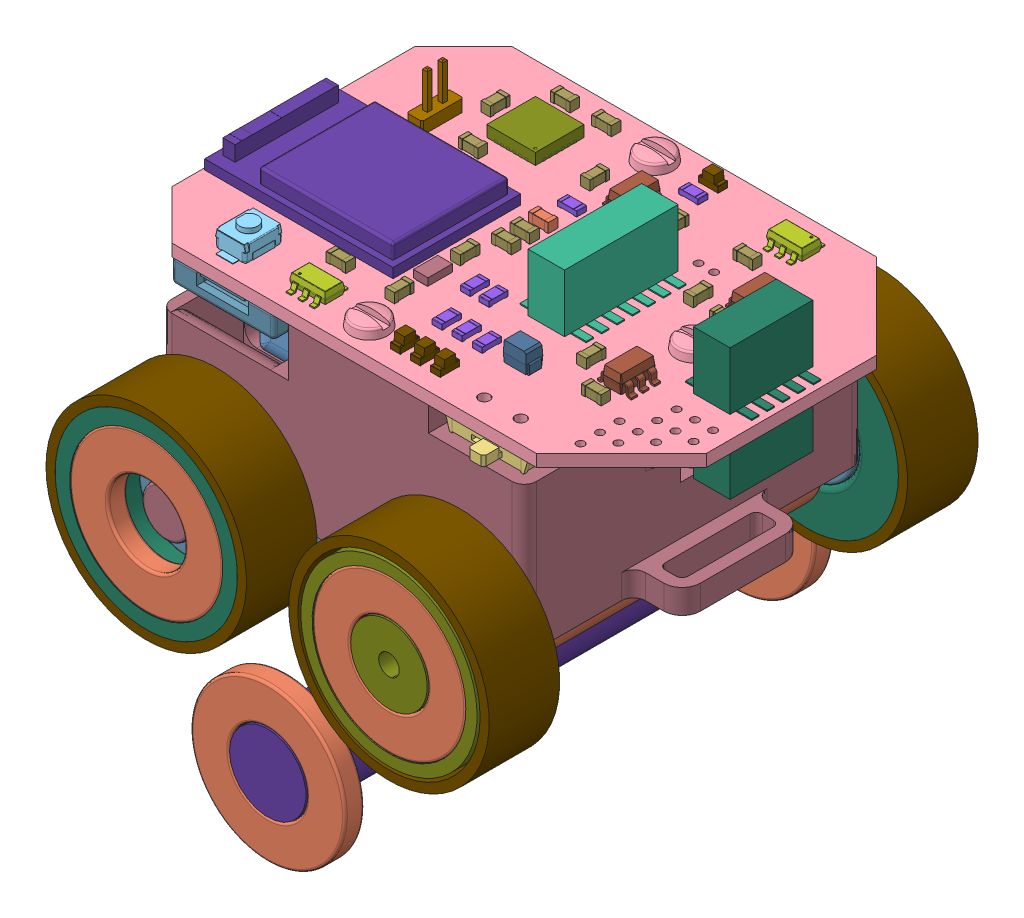
SolidWorks assembly AstroAnt_small_magnet, configuration Default. Lengths in mm.
Overall size (41.76 38.98 40.25).
158 component instances, 38 part files, 35 mates.
Components (placement in the parent):
- LiPo_360mAh-1: LiPo_360mAh [Default] at (6.8166 4.9998 44.2756) size (25 7 18)
- PA2-50-1: PA2-50 [Default] at (8.0673 -18.301 41.8029) x (0 0 1) z (0.952879 0.303349 0) size (29.1 8 8)
- PA2-50-2: PA2-50 [Default] at (-4.1563 19.5334 49.6029) x (0 0 -1) z (0.755989 -0.654584 0) size (29.1 8 8)
- 92120A150_Brass Heat-Set Inserts for Plastic-1: 92120A150_Brass Heat-Set Inserts for Plastic [92120A150] at (19.9543 12.4998 45.7029) size (2.56 3.33 2.56)
- 92120A150_Brass Heat-Set Inserts for Plastic-2: 92120A150_Brass Heat-Set Inserts for Plastic [92120A150] at (4.9543 12.4998 33.9529) size (2.56 3.33 2.56)
- 92120A150_Brass Heat-Set Inserts for Plastic-3: 92120A150_Brass Heat-Set Inserts for Plastic [92120A150] at (4.9543 12.4998 57.4529) size (2.56 3.33 2.56)
- 91460A005_METRIC CHEESE HEAD SLOTTED MACHINE SCREW-8: 91460A005_METRIC CHEESE HEAD SLOTTED MACHINE SCREW [91460A005] at (4.9543 14.9998 57.4529) x (1 0 0) z (0 1 0) size (3 3 7.1)
- 91460A005_METRIC CHEESE HEAD SLOTTED MACHINE SCREW-9: 91460A005_METRIC CHEESE HEAD SLOTTED MACHINE SCREW [91460A005] at (4.9543 14.9998 33.9529) x (1 0 0) z (0 1 0) size (3 3 7.1)
- 91460A005_METRIC CHEESE HEAD SLOTTED MACHINE SCREW-10: 91460A005_METRIC CHEESE HEAD SLOTTED MACHINE SCREW [91460A005] at (19.9543 14.9998 45.7029) x (1 0 0) z (0 1 0) size (3 3 7.1)
- 92120A150_Brass Heat-Set Inserts for Plastic-4: 92120A150_Brass Heat-Set Inserts for Plastic [92120A150] at (4.9543 1.4998 57.4529) x (-0.616962 0 -0.786993) z (0.786993 0 -0.616962) size (2.56 3.33 2.56)
- 92120A150_Brass Heat-Set Inserts for Plastic-5: 92120A150_Brass Heat-Set Inserts for Plastic [92120A150] at (4.9543 1.4998 33.9529) x (-0.616962 0 -0.786993) z (0.786993 0 -0.616962) size (2.56 3.33 2.56)
- 91460A005_METRIC CHEESE HEAD SLOTTED MACHINE SCREW-14: 91460A005_METRIC CHEESE HEAD SLOTTED MACHINE SCREW [91460A005] at (4.9543 -2.5002 57.4529) x (0.663599 0 0.748089) z (0 -1 0) size (3 3 7.1)
- 91460A005_METRIC CHEESE HEAD SLOTTED MACHINE SCREW-15: 91460A005_METRIC CHEESE HEAD SLOTTED MACHINE SCREW [91460A005] at (4.9543 -2.5002 33.9529) x (0.663599 0 0.748089) z (0 -1 0) size (3 3 7.1)
- mainboard_v1.step-1: mainboard_v1.step [Default] at (-103.0457 13.9998 235.7029) x (0 0 -1) z (0 1 0) size (29.41 41 10.8)
  - B3U-1000P.step-1: B3U-1000P.step [Default] at (178.95 -97.38 1.05) x (1 0 0) z (0 -1 0) size (4 1.75 2.5)
    - COMPOUND.step-1: COMPOUND.step [Default] at origin size (4 1.75 2.5)
  - 20021321-00014C1LF.step-1: 20021321-00014C1LF.step [Default] at (190 -115.5 1.05) size (9.35 5.45 4.85)
    - COMPOUND-0.step-1: COMPOUND-0.step [Default] at origin size (9.35 5.45 4.85)
  - MP6513GJ-Z.step-1: MP6513GJ-Z.step [Default] at (201.21 -120 1.05) x (-1 0 0) z (0 0 1) size (2.8 2.9 1)
    - COMPOUND-1.step-1: COMPOUND-1.step [Default] at origin size (2.8 2.9 1)
  - MP6513GJ-Z.step-2: MP6513GJ-Z.step [Default] at (178.51 -103.46 1.05) size (2.8 2.9 1)
    - COMPOUND-1.step-1: COMPOUND-1.step [Default] at origin size (2.8 2.9 1)
  - R_0603_1608Metric.step-1: R_0603_1608Metric.step [Default] at (195.55 -104.38 -0.05) x (1 0 0) z (0 0 -1) size (1.6 0.8 0.45)
    - SOLID.step-1: SOLID.step [Default] at origin size (1.6 0.8 0.45)
  - R_0603_1608Metric.step-2: R_0603_1608Metric.step [Default] at (192.6 -99.86 -0.05) x (0 1 0) z (0 0 -1) size (1.6 0.8 0.45)
    - SOLID.step-1: SOLID.step [Default] at origin size (1.6 0.8 0.45)
  - PinHeader_2x01_P1.27mm_Vertical.step-1: PinHeader_2x01_P1.27mm_Vertical.step [Default] at (194.96 -96.07 1.05) size (3.4 1.27 6.3)
    - SOLID-2.step-1: SOLID-2.step [Default] at origin size (3.4 1.27 6.3)
  - TAJP106K010RNJ.step-1: TAJP106K010RNJ.step [Default] at (196.22 -98.14 -0.05) x (-1 0 0) z (0 0 -1) size (2.05 1.4 1.7)
    - COMPOUND-3.step-1: COMPOUND-3.step [Default] at origin size (2.05 1.4 1.7)
  - TAJP106K010RNJ.step-2: TAJP106K010RNJ.step [Default] at (181.68 -117.23 1.05) x (0 1 0) z (0 0 1) size (2.05 1.4 1.7)
    - COMPOUND-3.step-1: COMPOUND-3.step [Default] at origin size (2.05 1.4 1.7)
  - SOT-23-5.step-1: SOT-23-5.step [Default] at (195.38 -122.78 1.05) x (0 1 0) z (0 0 1) size (2.8 2.9 1.55)
    - SOLID-4.step-1: SOLID-4.step [Default] at origin size (2.8 2.9 1.55)
  - C_0603_1608Metric.step-1: C_0603_1608Metric.step [Default] at (192.91 -122.55 1.05) x (0 -1 0) z (0 0 1) size (1.6 0.8 0.8)
    - SOLID-5.step-1: SOLID-5.step [Default] at origin size (1.6 0.8 0.8)
  - C_0603_1608Metric.step-2: C_0603_1608Metric.step [Default] at (193.57 -119.76 1.05) size (1.6 0.8 0.8)
    - SOLID-5.step-1: SOLID-5.step [Default] at origin size (1.6 0.8 0.8)
  - ECS-.327-12.5-12-TR.step-1: ECS-.327-12.5-12-TR.step [Default] at (184.31 -107.18 1.05) size (2 1.2 0.7)
    - COMPOUND-6.step-1: COMPOUND-6.step [Default] at origin size (2 1.2 0.7)
  - C_0603_1608Metric.step-3: C_0603_1608Metric.step [Default] at (197.67 -113.69 1.05) size (1.6 0.8 0.8)
    - SOLID-5.step-1: SOLID-5.step [Default] at origin size (1.6 0.8 0.8)
  - C_0603_1608Metric.step-4: C_0603_1608Metric.step [Default] at (197.64 -107.18 1.05) size (1.6 0.8 0.8)
    - SOLID-5.step-1: SOLID-5.step [Default] at origin size (1.6 0.8 0.8)
  - C_0603_1608Metric.step-5: C_0603_1608Metric.step [Default] at (190.96 -108.09 1.05) x (0 1 0) z (0 0 1) size (1.6 0.8 0.8)
    - SOLID-5.step-1: SOLID-5.step [Default] at origin size (1.6 0.8 0.8)
  - 1734592-6.step-1: 1734592-6.step [Default] at (203.79 -118 -1.05) x (0 -1 0) z (1 0 0) size (8.43 2.05 5.11)
    - SOLID-7.step-1: SOLID-7.step [Default] at origin size (8.43 2.05 5.11)
  - 1734592-6.step-2: 1734592-6.step [Default] at (176.19 -98 -1.05) x (0 1 0) z (-1 0 0) size (8.43 2.05 5.11)
    - SOLID-7.step-1: SOLID-7.step [Default] at origin size (8.43 2.05 5.11)
  - 20021321-00010C4LF.step-1: 20021321-00010C4LF.step [Default] at (190 -127.85 -0.05) x (1 0 0) z (0 0 -1) size (6.81 5.45 4.85)
    - COMPOUND-8.step-1: COMPOUND-8.step [Default] at origin size (6.81 5.45 4.85)
  - 20021321-00010C4LF.step-2: 20021321-00010C4LF.step [Default] at (190 -127.85 1.05) size (6.81 5.45 4.85)
    - COMPOUND-8.step-1: COMPOUND-8.step [Default] at origin size (6.81 5.45 4.85)
  - C_0603_1608Metric.step-6: C_0603_1608Metric.step [Default] at (181.31 -102.6 1.05) x (0 -1 0) z (0 0 1) size (1.6 0.8 0.8)
    - SOLID-5.step-1: SOLID-5.step [Default] at origin size (1.6 0.8 0.8)
  - C_0603_1608Metric.step-7: C_0603_1608Metric.step [Default] at (198.25 -119.14 1.05) x (0 -1 0) z (0 0 1) size (1.6 0.8 0.8)
    - SOLID-5.step-1: SOLID-5.step [Default] at origin size (1.6 0.8 0.8)
  - MPU6050.step-1: MPU6050.step [Default] at (198.43 -101.5 1.05) x (0 1 0) z (1 0 0) size (4 0.95 4)
    - COMPOUND-9.step-1: COMPOUND-9.step [Default] at origin size (4 0.95 4)
  - C_0603_1608Metric.step-8: C_0603_1608Metric.step [Default] at (194.9 -99.89 1.05) x (0 -1 0) z (0 0 1) size (1.6 0.8 0.8)
    - SOLID-5.step-1: SOLID-5.step [Default] at origin size (1.6 0.8 0.8)
  - C_0603_1608Metric.step-9: C_0603_1608Metric.step [Default] at (201.98 -100.38 1.05) x (0 -1 0) z (0 0 1) size (1.6 0.8 0.8)
    - SOLID-5.step-1: SOLID-5.step [Default] at origin size (1.6 0.8 0.8)
  - C_0603_1608Metric.step-10: C_0603_1608Metric.step [Default] at (201.98 -103.78 1.05) x (0 1 0) z (0 0 1) size (1.6 0.8 0.8)
    - SOLID-5.step-1: SOLID-5.step [Default] at origin size (1.6 0.8 0.8)
  - C_0603_1608Metric.step-11: C_0603_1608Metric.step [Default] at (198.81 -97.82 1.05) size (1.6 0.8 0.8)
    - SOLID-5.step-1: SOLID-5.step [Default] at origin size (1.6 0.8 0.8)
  - SOT-23-5.step-2: SOT-23-5.step [Default] at (184.86 -122.77 1.05) x (0 1 0) z (0 0 1) size (2.8 2.9 1.55)
    - SOLID-4.step-1: SOLID-4.step [Default] at origin size (2.8 2.9 1.55)
  - SOT-23-5.step-3: SOT-23-5.step [Default] at (197.58 -110.46 1.05) x (0 1 0) z (0 0 1) size (2.8 2.9 1.55)
    - SOLID-4.step-1: SOLID-4.step [Default] at origin size (2.8 2.9 1.55)
  - MDBT50Q-1MV2.step-1: MDBT50Q-1MV2.step [Default] at (187.3136 -98.605 1.0754) x (-1 0 0) z (0 1 0) size (10.5 2.06 15.5)
    - SOLID-10.step-1: SOLID-10.step [Default] at origin size (10.5 2.06 15.5)
  - C_0603_1608Metric.step-12: C_0603_1608Metric.step [Default] at (189.44 -108.09 1.05) x (0 1 0) z (0 0 1) size (1.6 0.8 0.8)
    - SOLID-5.step-1: SOLID-5.step [Default] at origin size (1.6 0.8 0.8)
  - C_0603_1608Metric.step-13: C_0603_1608Metric.step [Default] at (181.57 -107.18 1.05) x (-1 0 0) z (0 0 1) size (1.6 0.8 0.8)
    - SOLID-5.step-1: SOLID-5.step [Default] at origin size (1.6 0.8 0.8)
  - C_0603_1608Metric.step-14: C_0603_1608Metric.step [Default] at (186.97 -107.18 1.05) size (1.6 0.8 0.8)
    - SOLID-5.step-1: SOLID-5.step [Default] at origin size (1.6 0.8 0.8)
  - C_0603_1608Metric.step-15: C_0603_1608Metric.step [Default] at (184.77 -119.75 1.05) x (-1 0 0) z (0 0 1) size (1.6 0.8 0.8)
    - SOLID-5.step-1: SOLID-5.step [Default] at origin size (1.6 0.8 0.8)
  - C_0603_1608Metric.step-16: C_0603_1608Metric.step [Default] at (182.37 -122.54 1.05) x (0 -1 0) z (0 0 1) size (1.6 0.8 0.8)
    - SOLID-5.step-1: SOLID-5.step [Default] at origin size (1.6 0.8 0.8)
  - LED_0603_1608Metric.step-1: LED_0603_1608Metric.step [Default] at (178.19 -111.01 1.05) size (1.6 0.8 1.1)
    - SOLID-11.step-1: SOLID-11.step [Default] at origin size (1.6 0.8 1.1)
  - LED_0603_1608Metric.step-2: LED_0603_1608Metric.step [Default] at (178.19 -112.66 1.05) size (1.6 0.8 1.1)
    - SOLID-11.step-1: SOLID-11.step [Default] at origin size (1.6 0.8 1.1)
  - LED_0603_1608Metric.step-3: LED_0603_1608Metric.step [Default] at (178.19 -114.31 1.05) size (1.6 0.8 1.1)
    - SOLID-11.step-1: SOLID-11.step [Default] at origin size (1.6 0.8 1.1)
  - LED_0603_1608Metric.step-4: LED_0603_1608Metric.step [Default] at (202.34 -112.21 1.05) x (0 1 0) z (0 0 1) size (1.6 0.8 1.1)
    - SOLID-11.step-1: SOLID-11.step [Default] at origin size (1.6 0.8 1.1)
  - 473460001.step-1: 473460001.step [Default] at (201.68 -99.72 -1.25) x (0 -1 0) z (1 0 0) size (7.98 2.94 5.43)
    - COMPOUND-12.step-1: COMPOUND-12.step [Default] at origin size (7.98 2.94 5.43)
  - L_0603_1608Metric.step-1: L_0603_1608Metric.step [Default] at (192.48 -108.09 1.05) x (0 1 0) z (0 0 1) size (1.6 0.8 0.8)
    - SOLID-13.step-1: SOLID-13.step [Default] at origin size (1.6 0.8 0.8)
  - R_0603_1608Metric.step-3: R_0603_1608Metric.step [Default] at (185.18 -111.31 1.05) x (-1 0 0) z (0 0 1) size (1.6 0.8 0.45)
    - SOLID.step-1: SOLID.step [Default] at origin size (1.6 0.8 0.45)
  - R_0603_1608Metric.step-4: R_0603_1608Metric.step [Default] at (185.18 -109.77 1.05) size (1.6 0.8 0.45)
    - SOLID.step-1: SOLID.step [Default] at origin size (1.6 0.8 0.45)
  - R_0603_1608Metric.step-5: R_0603_1608Metric.step [Default] at (181.62 -111.01 1.05) size (1.6 0.8 0.45)
    - SOLID.step-1: SOLID.step [Default] at origin size (1.6 0.8 0.45)
  - R_0603_1608Metric.step-6: R_0603_1608Metric.step [Default] at (181.62 -112.66 1.05) size (1.6 0.8 0.45)
    - SOLID.step-1: SOLID.step [Default] at origin size (1.6 0.8 0.45)
  - R_0603_1608Metric.step-7: R_0603_1608Metric.step [Default] at (181.62 -114.31 1.05) x (-1 0 0) z (0 0 1) size (1.6 0.8 0.45)
    - SOLID.step-1: SOLID.step [Default] at origin size (1.6 0.8 0.45)
  - R_0603_1608Metric.step-8: R_0603_1608Metric.step [Default] at (194.84 -108.1 1.05) x (0 1 0) z (0 0 1) size (1.6 0.8 0.45)
    - SOLID.step-1: SOLID.step [Default] at origin size (1.6 0.8 0.45)
  - R_0603_1608Metric.step-9: R_0603_1608Metric.step [Default] at (200.69 -112.2325 1.05) x (0 1 0) z (0 0 1) size (1.6 0.8 0.45)
    - SOLID.step-1: SOLID.step [Default] at origin size (1.6 0.8 0.45)
  - R_0603_1608Metric.step-10: R_0603_1608Metric.step [Default] at (196.22 -101.51 -0.05) x (-1 0 0) z (0 0 -1) size (1.6 0.8 0.45)
    - SOLID.step-1: SOLID.step [Default] at origin size (1.6 0.8 0.45)
  - R_0603_1608Metric.step-11: R_0603_1608Metric.step [Default] at (196.22 -99.9725 -0.05) x (-1 0 0) z (0 0 -1) size (1.6 0.8 0.45)
    - SOLID.step-1: SOLID.step [Default] at origin size (1.6 0.8 0.45)
  - SW_SPDT_PCM12.step-1: SW_SPDT_PCM12.step [Default] at (178.18 -119.37 -0.05) x (0 1 0) z (0 0 -1) size (7.7 5 2)
    - SOLID-14.step-1: SOLID-14.step [Default] at origin size (7.7 5 2)
  - COMPOUND-15.step-1: COMPOUND-15.step [Default] at origin size (28 41 1)
- 91613A020_METRIC CHEESE HEAD SLOTTED MACHINE SCREW-1: 91613A020_METRIC CHEESE HEAD SLOTTED MACHINE SCREW [91613A020] at (1.2533 -0.5002 54.4029) x (1 0 0) z (0 1 0) size (3 3 5.08)
- 91613A020_METRIC CHEESE HEAD SLOTTED MACHINE SCREW-2: 91613A020_METRIC CHEESE HEAD SLOTTED MACHINE SCREW [91613A020] at (8.6533 -0.5002 54.4029) x (1 0 0) z (0 1 0) size (3 3 5.08)
- 91613A020_METRIC CHEESE HEAD SLOTTED MACHINE SCREW-3: 91613A020_METRIC CHEESE HEAD SLOTTED MACHINE SCREW [91613A020] at (1.2533 -0.5002 37.0029) x (1 0 0) z (0 1 0) size (3 3 5.08)
- IR_TEMP_V2.step-3: IR_TEMP_V2.step [Default] at (118.9553 -0.5002 109.7029) x (-1 0 0) z (0 1 0) size (10 20 4.8)
  - Board_Geoms_380f.step-1: Board_Geoms_380f.step [Default] at origin size (10 20 1.11)
    - Pcb_380f.step-1: Pcb_380f.step [Default] at origin size (10 20 1)
    - topTracks_380f.step-1: topTracks_380f.step [Default] at (0 0 0.01) size (9.62 17.53 0.05)
    - botTracks_380f.step-1: botTracks_380f.step [Default] at (0 0 -1.01) size (9.25 16.88 0.05)
  - Step_Models_380f.step-1: Step_Models_380f.step [Default] at origin size (9.46 10.17 4.8)
    - Top_380f.step-1: Top_380f.step [Default] at origin size (9.46 10.17 1.2)
      - IC1_PW14_613E6C6D.step-1: IC1_PW14_613E6C6D.step [Default] at (113.99 -59.48 0) x (-1 0 0) z (0 1 0) size (6.4 1.2 5)
      - C1_C_0402_1005Metric_613EDDF6.step-1: C1_C_0402_1005Metric_613EDDF6.step [Default] at (110.5 -64.26 0) x (-1 0 0) z (0 0 1) size (1 0.5 0.5)
      - C1_C_0402_1005Metric_613EDDF6.step-2: C1_C_0402_1005Metric_613EDDF6.step [Default] at (109.52 -61.07 0) x (0 -1 0) z (0 0 1) size (1 0.5 0.5)
      - C1_C_0402_1005Metric_613EDDF6.step-3: C1_C_0402_1005Metric_613EDDF6.step [Default] at (118.48 -60.86 0) x (0 -1 0) z (0 0 1) size (1 0.5 0.5)
      - C1_C_0402_1005Metric_613EDDF6.step-4: C1_C_0402_1005Metric_613EDDF6.step [Default] at (118.48 -58.59 0) x (0 -1 0) z (0 0 1) size (1 0.5 0.5)
      - C1_C_0402_1005Metric_613EDDF6.step-5: C1_C_0402_1005Metric_613EDDF6.step [Default] at (113.32 -66.9 0) size (1 0.5 0.5)
      - R1_R_0402_1005Metric_613EDE7A.step-1: R1_R_0402_1005Metric_613EDE7A.step [Default] at (110.98 -63.1 0) size (1 0.5 0.35)
      - R1_R_0402_1005Metric_613EDE7A.step-2: R1_R_0402_1005Metric_613EDE7A.step [Default] at (111.68 -66.3 0) x (0 1 0) z (0 0 1) size (1 0.5 0.35)
    - Bot_380f.step-1: Bot_380f.step [Default] at origin size (6.35 7.64 4.6)
      - U1_ZTP-135SR_613E6CD4.step-1: U1_ZTP-135SR_613E6CD4.step [Default] at (114 -64 -1) x (-1 0 0) z (0 -1 0) size (6.35 4.6 5.4)
      - C1_C_0402_1005Metric_613EDDF6.step-1: C1_C_0402_1005Metric_613EDDF6.step [Default] at (115.07 -59.56 -1) x (0 -1 0) z (0 0 -1) size (1 0.5 0.5)
      - R1_R_0402_1005Metric_613EDE7A.step-1: R1_R_0402_1005Metric_613EDE7A.step [Default] at (113.64 -59.58 -1) x (0 -1 0) z (0 0 -1) size (1 0.5 0.35)
- Body_simple-1: Body_simple [Default] at (4.8007 -0.0002 38.7677) size (34 16 37)
- ball_bearing_5x11x4mm-1: ball_bearing_5x11x4mm [Default] at (-45.4624 -2.1758 28.9029) x (0.999925 -0.012245 0) z (0 0 1) size (8 8 2.5)
- wheel_holder_non_motor-1: wheel_holder_non_motor [Default] at (-70.2522 1.7638 25.6029) size (15 15 5.8)
- wheel_holder_non_motor-2: wheel_holder_non_motor [Default] at (-19.1131 -84.0559 65.8029) x (0.185441 0.982655 0) z (0 0 -1) size (15 15 5.8)
- ball_bearing_5x11x4mm-2: ball_bearing_5x11x4mm [Default] at (-30.2803 -54.9376 62.5029) x (0.373101 0.927791 0) z (0 0 -1) size (8 8 2.5)
- wheel_motor-1: wheel_motor [Default] at (24.0366 1.7037 25.5779) size (14.5 14.5 5.8)
- wheel_motor-2: wheel_motor [Default] at (15.5431 29.126 65.8279) x (-0.038296 0.999266 0) z (0 0 -1) size (14.5 14.5 5.8)
- magnet_wheel_holder-1: magnet_wheel_holder [Default] at (28.927 0.8494 25.6029) size (6.3 6.3 40.2)
- tire-1: tire [Default] at (38.167 -1.442 25.5779) size (16.5 16.5 5.8)
- tire-2: tire [Default] at (58.167 -1.442 25.6029) size (16.5 16.5 5.8)
- tire-3: tire [Default] at (38.167 -1.442 60.0029) size (16.5 16.5 5.8)
- tire-4: tire [Default] at (58.167 -1.442 60.0279) size (16.5 16.5 5.8)
- motor_holder-2: motor_holder [Default] at (-0.192 -4.0002 11.9282) size (20 4.13 28)
- R8201-1: R8201 [Default] at (-53.4439 -3.2146 25.6029) size (12.7 12.7 1.59)
- R8201-2: R8201 [Default] at (-73.4439 -3.2146 25.5779) size (12.7 12.7 1.59)
- R8201-3: R8201 [Default] at (-53.4439 -3.2146 64.2404) size (12.7 12.7 1.59)
- R8201-4: R8201 [Default] at (-73.4439 -3.2146 64.2154) size (12.7 12.7 1.59)
- R8201-5: R8201 [Default] at (-63.4439 -15.9439 25.6029) size (12.7 12.7 1.59)
- R8201-6: R8201 [Default] at (-63.4439 -15.9439 64.2154) size (12.7 12.7 1.59)
Mates (geometry in assembly coordinates):
- Coincident100: coincident anti-aligned: plane of mainboard_v1.step-1/COMPOUND-15.step-1 through (6.7692 13.9998 45.7029) normal (0 -1 0); plane of Body_simple-1 through (4.8007 13.9998 38.7677) normal (0 1 0)
- Concentric58: concentric anti-aligned: cylinder of PA2-50-2 through (-5.0457 -0.0002 33.4029) axis (0 0 1) radius 4; cylinder of Body_simple-1 through (-5.0457 -0.0002 57.7029) axis (0 0 -1) radius 4.1
- Concentric59: concentric aligned: cylinder of mainboard_v1.step-1/COMPOUND-15.step-1 through (19.9543 13.4998 45.7029) axis (0 1 0) radius 0.85; cylinder of Body_simple-1 through (19.9543 5.9998 45.7029) axis (0 1 0) radius 1.15
- Concentric63: concentric anti-aligned: cylinder of ball_bearing_5x11x4mm-1 through (14.9543 -0.0002 31.4029) axis (0 0 -1) radius 4; cylinder of wheel_holder_non_motor-1 through (14.9543 -0.0002 25.6029) axis (0 0 1) radius 4
- Concentric66: concentric anti-aligned: cylinder of Body_simple-1 through (14.9543 -0.0002 27.2029) axis (0 0 1) radius 2; cylinder of ball_bearing_5x11x4mm-1 through (14.9543 -0.0002 32.9029) axis (0 0 -1) radius 2
- Distance2: distance = 0.3 mm anti-aligned: plane of wheel_holder_non_motor-1 through (14.9543 -0.0002 31.4029) normal (0 0 1); plane of Body_simple-1 through (-10.0457 13.9998 31.7029) normal (0 0 -1)
- Coincident105: coincident aligned: plane of ball_bearing_5x11x4mm-1 through (14.9543 -0.0002 31.4029) normal (0 0 1); plane of wheel_holder_non_motor-1 through (14.9543 -0.0002 31.4029) normal (0 0 1)
- Distance3: distance = 0.3 mm anti-aligned: plane of wheel_holder_non_motor-2 through (-5.0457 -0.0002 60.0029) normal (0 0 -1); plane of Body_simple-1 through (-10.0457 13.9998 59.7029) normal (0 0 1)
- Concentric67: concentric aligned: cylinder of Body_simple-1 through (-5.0457 -0.0002 64.2029) axis (0 0 -1) radius 2; cylinder of wheel_holder_non_motor-2 through (-5.0457 -0.0002 65.8029) axis (0 0 -1) radius 4
- Coincident107: coincident aligned: plane of wheel_holder_non_motor-2 through (-5.0457 -0.0002 60.0029) normal (0 0 -1); plane of ball_bearing_5x11x4mm-2 through (-5.0457 -0.0002 60.0029) normal (0 0 -1)
- Concentric68: concentric anti-aligned: cylinder of Body_simple-1 through (-5.0457 -0.0002 64.2029) axis (0 0 -1) radius 2; cylinder of ball_bearing_5x11x4mm-2 through (-5.0457 -0.0002 58.5029) axis (0 0 1) radius 2
- Concentric83: concentric anti-aligned: cylinder of wheel_motor-1 through (-5.0457 -0.0002 31.3779) axis (0 0 -1) radius 7.25; cylinder of tire-1 through (-5.0457 -0.0002 25.5779) axis (0 0 1) radius 7.5
- Coincident123: coincident aligned: plane of wheel_motor-1 through (-5.0457 -0.0002 25.5779) normal (0 0 -1); plane of tire-1 through (-5.0457 -0.0002 25.5779) normal (0 0 -1)
- Concentric84: concentric anti-aligned: cylinder of wheel_holder_non_motor-1 through (14.9543 -0.0002 31.4029) axis (0 0 -1) radius 7.5; cylinder of tire-2 through (14.9543 -0.0002 25.6029) axis (0 0 1) radius 7.5
- Coincident124: coincident aligned: plane of wheel_holder_non_motor-1 through (14.9543 -0.0002 25.6029) normal (0 0 -1); plane of tire-2 through (14.9543 -0.0002 25.6029) normal (0 0 -1)
- Coincident125: coincident aligned: plane of wheel_motor-2 through (14.9543 -0.0002 65.8279) normal (0 0 1); plane of tire-4 through (14.9543 -0.0002 65.8279) normal (0 0 1)
- Concentric85: concentric aligned: cylinder of wheel_motor-2 through (14.9543 -0.0002 60.0279) axis (0 0 1) radius 7.25; cylinder of tire-4 through (14.9543 -0.0002 60.0279) axis (0 0 1) radius 7.5
- Coincident126: coincident aligned: plane of wheel_holder_non_motor-2 through (-5.0457 -0.0002 65.8029) normal (0 0 1); plane of tire-3 through (-5.0457 -0.0002 65.8029) normal (0 0 1)
- Concentric86: concentric aligned: cylinder of wheel_holder_non_motor-2 through (-5.0457 -0.0002 60.0029) axis (0 0 1) radius 7.5; cylinder of tire-3 through (-5.0457 -0.0002 60.0029) axis (0 0 1) radius 7.5
- Concentric94: concentric anti-aligned: cylinder of IR_TEMP_V2.step-3/Step_Models_380f.step-1/Bot_380f.step-1/U1_ZTP-135SR_613E6CD4.step-1 through (4.9553 -4.1002 45.7029) axis (0 1 0) radius 2.35; cylinder of motor_holder-2 through (4.9553 -0.0002 45.7029) axis (0 -1 0) radius 4.15
- Coincident128: coincident anti-aligned: plane of IR_TEMP_V2.step-3/Board_Geoms_380f.step-1/Pcb_380f.step-1 through (4.9553 -1.5002 45.7029) normal (0 -1 0); plane of motor_holder-2 through (-0.192 -1.5002 11.9282) normal (0 1 0)
- Concentric95: concentric anti-aligned: cylinder of Body_simple-1 through (14.9543 -0.0002 27.2029) axis (0 0 1) radius 2; cylinder of R8201-1 through (14.9543 -0.0002 27.1904) axis (0 0 -1) radius 3.175
- Concentric96: concentric aligned: cylinder of wheel_motor-1 through (-5.0457 -0.0002 28.5779) axis (0 0 -1) radius 3.15; cylinder of R8201-2 through (-5.0457 -0.0002 27.1654) axis (0 0 -1) radius 3.175
- Concentric97: concentric anti-aligned: cylinder of wheel_motor-2 through (14.9543 -0.0002 62.8279) axis (0 0 1) radius 3.15; cylinder of R8201-3 through (14.9543 -0.0002 65.8279) axis (0 0 -1) radius 3.175
- Concentric98: concentric aligned: cylinder of Body_simple-1 through (-5.0457 -0.0002 64.2029) axis (0 0 -1) radius 2; cylinder of R8201-4 through (-5.0457 -0.0002 65.8029) axis (0 0 -1) radius 3.175
- Coincident130: coincident aligned: plane of wheel_holder_non_motor-2 through (-5.0457 -0.0002 65.8029) normal (0 0 1); plane of R8201-4 through (-5.0457 -0.0002 65.8029) normal (0 0 1)
- Coincident131: coincident aligned: plane of wheel_motor-1 through (-5.0457 -0.0002 25.5779) normal (0 0 -1); plane of R8201-2 through (-5.0457 -0.0002 25.5779) normal (0 0 -1)
- Coincident132: coincident aligned: plane of wheel_holder_non_motor-1 through (14.9543 -0.0002 25.6029) normal (0 0 -1); plane of R8201-1 through (14.9543 -0.0002 25.6029) normal (0 0 -1)
- Concentric99: concentric anti-aligned: cylinder of PA2-50-1 through (14.9543 -0.0002 63.1029) axis (0 0 -1) radius 0.5; cylinder of wheel_motor-2 through (14.9543 -0.0002 60.0279) axis (0 0 1) radius 0.85
- Concentric100: concentric anti-aligned: cylinder of PA2-50-2 through (-5.0457 -0.0002 28.3029) axis (0 0 1) radius 0.5; cylinder of wheel_motor-1 through (-5.0457 -0.0002 31.3779) axis (0 0 -1) radius 0.85
- Coincident133: coincident aligned: plane of wheel_holder_non_motor-1 through (14.9543 -0.0002 25.6029) normal (0 0 -1); plane of R8201-5 through (4.9543 -12.7295 25.6029) normal (0 0 -1)
- Coincident134: coincident aligned: plane of wheel_holder_non_motor-2 through (-5.0457 -0.0002 65.8029) normal (0 0 1); plane of R8201-6 through (4.9543 -12.7295 65.8029) normal (0 0 1)
- Coincident135: coincident aligned: plane of wheel_motor-2 through (14.9543 -0.0002 65.8279) normal (0 0 1); plane of R8201-3 through (14.9543 -0.0002 65.8279) normal (0 0 1)
- Coincident136: coincident aligned: plane of magnet_wheel_holder-1 through (4.9543 -12.7295 65.8029) normal (0 0 1); plane of R8201-6 through (4.9543 -12.7295 65.8029) normal (0 0 1)
- Concentric101: concentric aligned: cylinder of magnet_wheel_holder-1 through (4.9543 -12.7295 65.8029) axis (0 0 -1) radius 3.15; cylinder of R8201-6 through (4.9543 -12.7295 65.8029) axis (0 0 -1) radius 3.175
